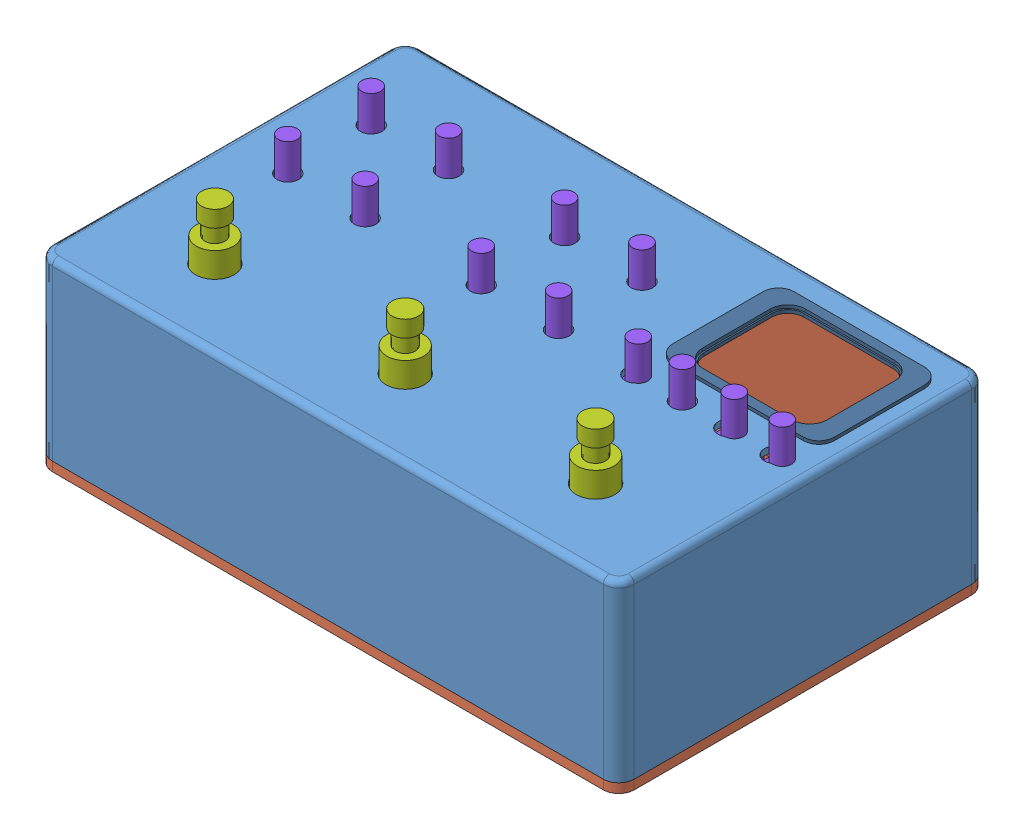
SolidWorks assembly 装配体203, configuration 默认. Lengths in mm.
Overall size (188 77.7 121).
25 component instances, 11 part files, 49 mates.
Components (placement in the parent):
- 壳体-1: 壳体 [默认] at (18.7461 20.6381 -2.5527) size (188 56.5 119)
- 底板-1: 底板 [默认] at (106.965 20.6381 -84.8282) x (-1 0 0) z (0 0 1) size (188 6 119)
- 2-1板卡-1: 2-1板卡 [默认] at (-15.4479 26.6681 48.4999) x (1 0 0) z (0 1 0) size (119.97 69.97 18.63)
- 音频口-1: 音频口 [默认] at (96.5561 48.8881 -54.5) x (-0.999999 -0.001298 0) z (0.001298 -0.999999 0) size (19 32 19)
- 音频口-2: 音频口 [默认] at (56.5561 48.8881 -54.5) x (-0.383049 0.923728 0) z (-0.923728 -0.383049 0) size (19 32 19)
- 耳机母座-1: 耳机母座 [默认] at (4.9626 48.2273 -71.9424) x (0 0 -1) z (0.923728 0.383049 0) size (26.5 8.1 8.1)
- DC头-1: DC头 [默认] at (-40.0511 48.8881 -39.3412) x (0 0 1) z (-1 0 0) size (31.5 12.5 12.5)
- 新踩钉-1: 新踩钉 [默认] at (88.0561 75.1381 34.5) x (0.999745 0 0.022577) z (-0.022577 0 0.999745) size (13 33.1 30.5)
- 新踩钉-2: 新踩钉 [默认] at (-34.9439 75.1381 34.5) size (13 33.1 30.5)
- 新踩钉-3: 新踩钉 [默认] at (26.5561 75.1381 34.5) size (13 33.1 30.5)
- 旋钮-1: 旋钮 [默认] at (7.8348 60.049 -2.5527) x (0 -1 0) z (0 0 1) size (28.5 11.1 11)
- 旋钮-4: 旋钮 [默认] at (105.0848 60.049 -2.5527) x (0 -1 0) z (0 0 1) size (28.5 11.1 11)
- 旋钮-5: 旋钮 [默认] at (32.8348 60.049 -29.5) x (0 -1 0) z (0 0 1) size (28.5 11.1 11)
- 旋钮-6: 旋钮 [默认] at (-29.6652 60.049 -29.5) x (0 -1 0) z (0 0 1) size (28.5 11.1 11)
- 旋钮-7: 旋钮 [默认] at (-54.6652 60.049 -29.5) x (0 -1 0) z (0 0 1) size (28.5 11.1 11)
- 旋钮-8: 旋钮 [默认] at (58.5848 60.049 -2.5527) x (0 -1 0) z (0 0 1) size (28.5 11.1 11)
- 旋钮-9: 旋钮 [默认] at (-29.6652 60.049 -2.5527) x (0 -1 0) z (0 0 1) size (28.5 11.1 11)
- 旋钮-11: 旋钮 [默认] at (72.8348 60.049 -2.5527) x (0 -1 0) z (0 0 1) size (28.5 11.1 11)
- 旋钮-12: 旋钮 [默认] at (7.8348 60.049 -29.5) x (0 -1 0) z (0 0 1) size (28.5 11.1 11)
- 旋钮-13: 旋钮 [默认] at (89.5848 60.049 -2.5527) x (0 -1 0) z (0 0 1) size (28.5 11.1 11)
- 旋钮-14: 旋钮 [默认] at (32.8348 60.049 -2.5527) x (0 -1 0) z (0 0 1) size (28.5 11.1 11)
- 旋钮-15: 旋钮 [默认] at (-54.6652 60.049 -2.5527) x (0 -1 0) z (0 0 1) size (28.5 11.1 11)
- usb选项-1: usb选项 [默认] at (-12.6125 48.8881 -56.5) x (1 0 0) z (0 -1 0) size (26.31 34 9.31)
- 屏幕扣-1: 屏幕扣 [默认] at (86.4443 77.1381 -28.4417) x (0 0 -1) z (-1 0 0) size (39.2 3.5 52.23)
- 屏幕-1: 屏幕 [默认] at (94.8549 73.4381 -31.6132) x (0 0 1) z (-1 0 0) size (32.2 3 49.23)
Mates (geometry in assembly coordinates):
- 重合1: coincident anti-aligned: plane of 壳体-1 through (18.7461 20.6381 -2.5527) normal (0 -1 0); plane of 底板-1 through (106.965 20.6381 -84.8282) normal (0 1 0)
- 同心1: concentric aligned: cylinder of 壳体-1 through (115.0561 40.6381 54) axis (0 -1 0) radius 2.25; circle of 底板-1
- 同心3: concentric aligned: cylinder of 壳体-1 through (-61.9439 40.6381 54) axis (0 -1 0) radius 2.25; circle of 底板-1
- 重合2: coincident anti-aligned: plane of 底板-1 through (106.965 20.6381 -84.8282) normal (0 1 0); plane of 2-1板卡-1 through (100.5563 20.6381 44.5001) normal (0 -1 0)
- 重合11: coincident anti-aligned: plane of 壳体-1 through (18.7461 269.3646 -56.5) normal (0 0 1); circle of 耳机母座-1
- 重合12: coincident anti-aligned: plane of 壳体-1 through (-67.4439 77.1381 -59.5) normal (0 0 -1); plane of DC头-1 through (-40.0511 48.8881 -59.5) normal (0 0 1)
- 重合13: coincident anti-aligned: plane of 壳体-1 through (112.5561 75.1381 -51.5) normal (0 -1 0); plane of 新踩钉-1 through (88.0561 75.1381 34.5) normal (0 1 0)
- 重合14: coincident anti-aligned: plane of 壳体-1 through (112.5561 75.1381 -51.5) normal (0 -1 0); plane of 新踩钉-3 through (26.5561 75.1381 34.5) normal (0 1 0)
- 重合15: coincident anti-aligned: plane of 壳体-1 through (112.5561 75.1381 -51.5) normal (0 -1 0); plane of 新踩钉-2 through (-34.9439 75.1381 34.5) normal (0 1 0)
- 重合16: coincident anti-aligned: plane of 壳体-1 through (112.5561 75.1381 -51.5) normal (0 -1 0); plane of 旋钮-6 through (-18.5652 75.1381 -34.2985) normal (0 1 0)
- 重合17: coincident anti-aligned: plane of 壳体-1 through (112.5561 75.1381 -51.5) normal (0 -1 0); plane of 旋钮-1 through (18.9348 75.1381 -7.3512) normal (0 1 0)
- 重合18: coincident anti-aligned: plane of 壳体-1 through (112.5561 75.1381 -51.5) normal (0 -1 0); plane of 旋钮-9 through (-18.5652 75.1381 -7.3512) normal (0 1 0)
- 重合20: coincident anti-aligned: plane of 壳体-1 through (112.5561 75.1381 -51.5) normal (0 -1 0); plane of 旋钮-15 through (-43.5652 75.1381 -7.3512) normal (0 1 0)
- 重合22: coincident anti-aligned: plane of 壳体-1 through (112.5561 75.1381 -51.5) normal (0 -1 0); plane of 旋钮-13 through (100.6848 75.1381 -7.3512) normal (0 1 0)
- 重合23: coincident anti-aligned: plane of 壳体-1 through (112.5561 75.1381 -51.5) normal (0 -1 0); plane of 旋钮-7 through (-43.5652 75.1381 -34.2985) normal (0 1 0)
- 重合24: coincident anti-aligned: plane of 壳体-1 through (112.5561 75.1381 -51.5) normal (0 -1 0); plane of 旋钮-4 through (116.1848 75.1381 -7.3512) normal (0 1 0)
- 重合26: coincident anti-aligned: plane of 壳体-1 through (112.5561 75.1381 -51.5) normal (0 -1 0); plane of 旋钮-11 through (83.9348 75.1381 -7.3512) normal (0 1 0)
- 重合28: coincident anti-aligned: plane of 壳体-1 through (112.5561 75.1381 -51.5) normal (0 -1 0); plane of 旋钮-5 through (43.9348 75.1381 -34.2985) normal (0 1 0)
- 重合29: coincident anti-aligned: plane of 壳体-1 through (112.5561 75.1381 -51.5) normal (0 -1 0); plane of 旋钮-8 through (69.6848 75.1381 -7.3512) normal (0 1 0)
- 重合30: coincident anti-aligned: plane of 壳体-1 through (112.5561 75.1381 -51.5) normal (0 -1 0); plane of 旋钮-14 through (43.9348 75.1381 -7.3512) normal (0 1 0)
- 同心15: concentric anti-aligned: circle of 壳体-1; cylinder of 旋钮-15 through (-48.4439 65.1381 -2.5527) axis (0 -1 0) radius 3.05
- 同心16: concentric anti-aligned: circle of 壳体-1; cylinder of 旋钮-6 through (-23.4439 88.1381 -29.5) axis (0 -1 0) radius 3.05
- 同心17: concentric anti-aligned: circle of 壳体-1; cylinder of 旋钮-9 through (-23.4439 65.1381 -2.5527) axis (0 -1 0) radius 3.05
- 同心19: concentric anti-aligned: circle of 壳体-1; cylinder of 旋钮-1 through (14.0561 65.1381 -2.5527) axis (0 -1 0) radius 3.05
- 同心20: concentric aligned: cylinder of 壳体-1 through (39.0561 77.1381 -2.5527) axis (0 -1 0) radius 3.5; cylinder of 旋钮-14 through (39.0561 88.1381 -2.5527) axis (0 -1 0) radius 3.05
- 同心21: concentric aligned: cylinder of 壳体-1 through (39.0561 77.1381 -29.5) axis (0 -1 0) radius 3.5; cylinder of 旋钮-5 through (39.0561 88.1381 -29.5) axis (0 -1 0) radius 3.05
- 同心22: concentric anti-aligned: circle of 壳体-1; cylinder of 旋钮-8 through (64.8061 65.1381 -2.5527) axis (0 -1 0) radius 3.05
- 同心23: concentric anti-aligned: circle of 壳体-1; cylinder of 旋钮-11 through (79.0561 88.1381 -2.5527) axis (0 -1 0) radius 3.05
- 同心24: concentric anti-aligned: circle of 壳体-1; cylinder of 旋钮-13 through (95.8061 65.1381 -2.5527) axis (0 -1 0) radius 3.05
- 同心25: concentric anti-aligned: circle of 壳体-1; cylinder of 旋钮-4 through (111.3061 65.1381 -2.5527) axis (0 -1 0) radius 3.05
- 同心26: concentric anti-aligned: circle of 壳体-1; cylinder of 旋钮-7 through (-48.4439 88.1381 -29.5) axis (0 -1 0) radius 3.05
- 重合32: coincident anti-aligned: plane of 壳体-1 through (18.7461 269.3646 -56.5) normal (0 0 1); plane of usb选项-1 through (-4.9439 36.3881 -56.5) normal (0 0 -1)
- 同心27: concentric aligned: cylinder of 壳体-1 through (-21.9439 48.8881 -39.5) axis (0 0 -1) radius 1.75; cylinder of usb选项-1 through (-21.9439 48.8881 -53.5) axis (0 0 -1) radius 1.5
- 同心28: concentric aligned: cylinder of 壳体-1 through (96.5561 48.8881 -39.5) axis (0 0 -1) radius 5.5; cylinder of 音频口-1 through (96.5561 48.8881 -29.5) axis (0 0 -1) radius 9.5
- 重合33: coincident anti-aligned: plane of 壳体-1 through (18.7461 269.3646 -56.5) normal (0 0 1); plane of 音频口-1 through (96.5561 36.3881 -56.5) normal (0 0 -1)
- 同心29: concentric aligned: circle of 壳体-1; cylinder of 音频口-2 through (56.5561 48.8881 -54.5) axis (0 0 -1) radius 3.25
- 重合34: coincident anti-aligned: plane of 壳体-1 through (18.7461 269.3646 -56.5) normal (0 0 1); plane of 音频口-2 through (56.5561 36.3881 -56.5) normal (0 0 -1)
- 同心30: concentric anti-aligned: cylinder of 底板-1 through (-11.4439 5.6381 -17.5) axis (0 1 0) radius 1.75; cylinder of 2-1板卡-1 through (-11.4439 28.1681 -17.5) axis (0 -1 0) radius 1.3
- 重合35: coincident anti-aligned: plane of 壳体-1 through (18.7461 77.1381 -2.5527) normal (0 1 0); plane of 屏幕扣-1 through (86.4443 77.1381 -28.4417) normal (0 -1 0)
- 平行4: parallel anti-aligned: line of 壳体-1 through (67.1911 77.1381 -12.55) axis (1 0 0); line of 屏幕扣-1 through (113.1711 74.6381 -12.55) axis (-1 0 0)
- 重合38: coincident anti-aligned: plane of 壳体-1 through (67.1911 74.1381 -12.55) normal (0 0 -1); plane of 屏幕扣-1 through (86.4443 74.6381 -12.55) normal (0 0 1)
- 重合39: coincident anti-aligned: plane of 壳体-1 through (113.1711 74.1381 -16.8) normal (-1 0 0); plane of 屏幕扣-1 through (113.1711 74.6381 -28.4417) normal (1 0 0)
- 同心34: concentric aligned: cylinder of 屏幕扣-1 through (111.1711 74.6381 -16.55) axis (0 1 0) radius 1; cylinder of 屏幕-1 through (111.1711 72.8381 -16.55) axis (0 1 0) radius 1.75
- 同心35: concentric aligned: cylinder of 屏幕扣-1 through (111.1711 74.6381 -44.75) axis (0 1 0) radius 1; circle of 屏幕-1
- 重合42: coincident anti-aligned: plane of 屏幕扣-1 through (86.4443 74.6381 -28.4417) normal (0 -1 0); plane of 屏幕-1 through (94.8549 74.6381 -31.6132) normal (0 1 0)
- 同心37: concentric aligned: cylinder of 壳体-1 through (6.5561 48.8881 -39.5) axis (0 0 -1) radius 3; cylinder of 耳机母座-1 through (6.5561 48.8881 -61.5) axis (0 0 -1) radius 2.75
- 同心38: concentric anti-aligned: cylinder of 壳体-1 through (-43.4439 48.8881 -39.5) axis (0 0 -1) radius 5.5; cylinder of DC头-1 through (-43.4439 48.8881 -30) axis (0 0 1) radius 6.25
- 同心39: concentric aligned: circle of 壳体-1; cylinder of 旋钮-12 through (14.0561 88.1381 -29.5) axis (0 -1 0) radius 3.05
- 重合43: coincident aligned: plane of 旋钮-5 through (43.9348 75.1381 -34.2985) normal (0 1 0); plane of 旋钮-12 through (18.9348 75.1381 -34.2985) normal (0 1 0)
